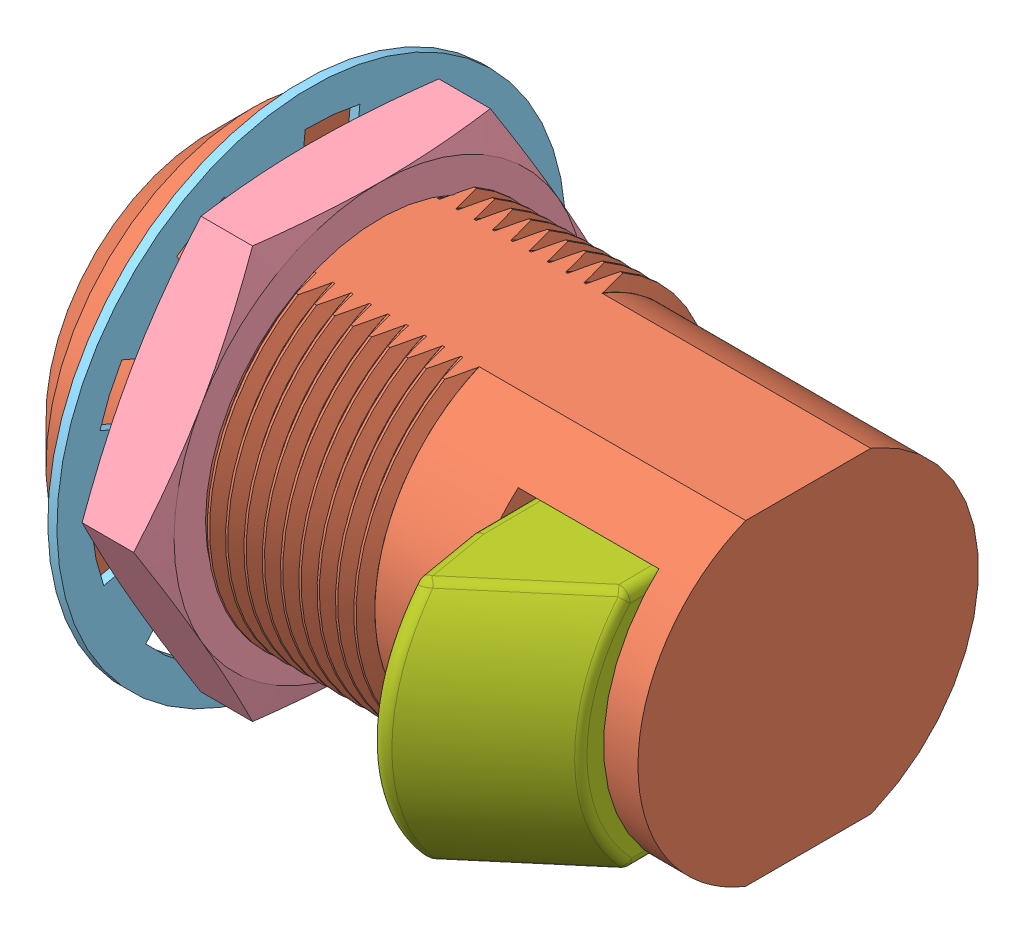
SolidWorks assembly Porte_Serrure_Cle, configuration Défaut. Lengths in mm.
Overall size (41.58 38.56 38.97).
7 component instances, 7 part files, 0 mates.
Components (placement in the parent):
- Porte_Serrure_Ressort-1: Porte_Serrure_Ressort [Défaut] at (-1.4058 10.243 9.1044) x (0 0 -1) z (1 0 0) size (21.49 4.59 4.57)
- Porte_Serrure_Support-1: Porte_Serrure_Support [Défaut] at (-26.6815 11.1833 12.473) x (-1 0 0) z (0 -1 0) size (41.46 28.7 28.7)
- Porte_Serrure_Insert_Cle-1: Porte_Serrure_Insert_Cle [Défaut] at (26.379 -212.8643 14.6) x (-1 0 0) z (0 0 -1) size (23.33 15.95 15.95)
- Porte_Serrure_Ecrou_Hex-1: Porte_Serrure_Ecrou_Hex [Défaut] at (-26.3115 -31.157 8.2014) x (0 0 1) z (-1 0 0) size (33 28.58 4.76)
- Porte_Serrure_Rondelle_Ecrou-1: Porte_Serrure_Rondelle_Ecrou [Défaut] at (-31.074 17.7899 -9.8703) x (0 0.096744 0.995309) z (-1 0 0) size (35.31 35.31 0.64)
- Porte_Serrure_Came-1: Porte_Serrure_Came [Défaut] at (-18.246 14.5659 16.3878) x (0 -1 0) z (1 0 0) size (12.45 12.01 13.54)
- Porte_Serrure_Pene-1: Porte_Serrure_Pene [Défaut] at (1.0072 5.2825 -10.1896) x (0 -0.999973 -0.007317) z (-1 0 0) size (16.91 23.47 9.63)
